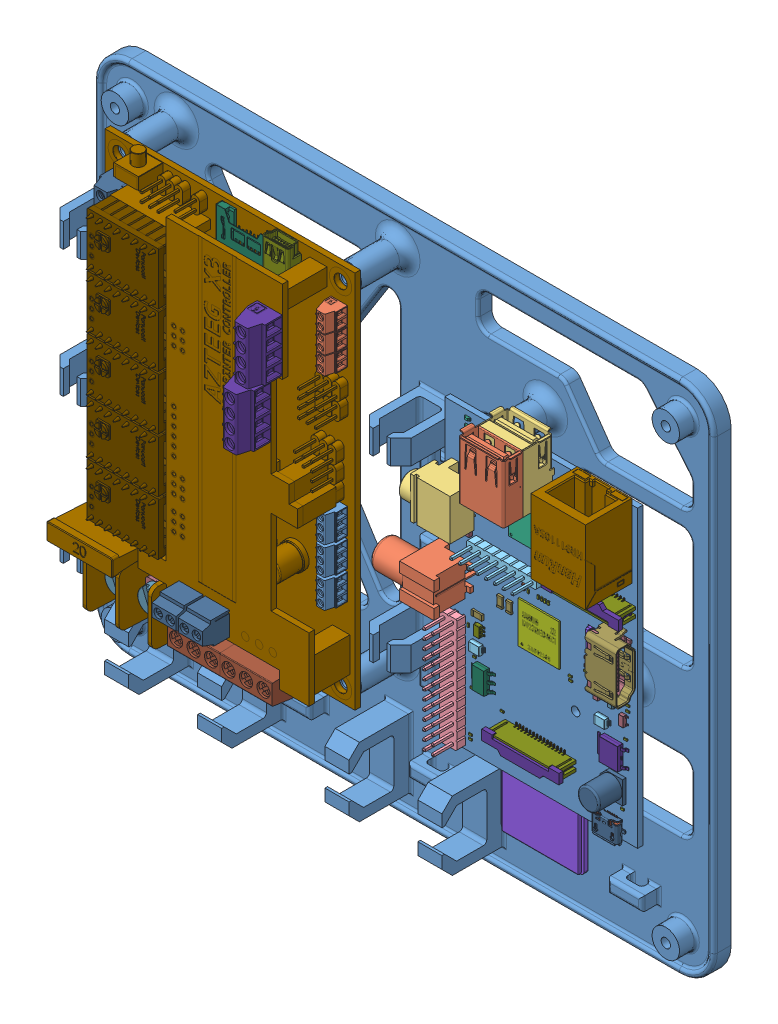
SolidWorks assembly Electronics_Package2, configuration Default. Lengths in mm.
Overall size (180 150 42.6).
296 component instances, 56 part files, 6 mates.
Components (placement in the parent):
- Electronics_Mount-1: Electronics_Mount [Default] at origin size (180 150 22)
- PARASOLID_raspberrypi_b_assembly_mounting_holes-1: PARASOLID_raspberrypi_b_assembly_mounting_holes [Default] at (55.4 9.4 19) x (0 1 0) z (0 0 1) size (110.83 65.9 20.48)
  - raspberry_pi__USB_x2-1: raspberry_pi__USB_x2 [Default] at (41.25 117.3116 21.0675) x (0 1 0) z (1 0 0) size (14.7 17.85 17.4)
    - raspberry_pi__USB_x2_part1-1: raspberry_pi__USB_x2_part1 [Default] at (-114.6616 -10.9375 -4.85) x (0 0 1) z (-1 0 0) size (17.4 6.35 14.7)
    - raspberry_pi__USB_x2_part2-1: raspberry_pi__USB_x2_part2 [Default] at (-114.6616 -19.4375 -4.85) x (0 0 1) z (-1 0 0) size (17.4 11.5 14.7)
  - raspberry_pi__SD_reader_assembly-1: raspberry_pi__SD_reader_assembly [Default] at (-46.9946 70.3951 -2.1406) x (0 1 0) z (-1 0 0) size (32.3 4.2 18.72)
    - raspberry_pi__SD_reader_body-1: raspberry_pi__SD_reader_body [Default] at (-67.8965 -2.1406 21.2643) size (32.3 4.2 16.75)
    - raspberry_pi__SD_reader_pin1-1: raspberry_pi__SD_reader_pin1 [Default] at (-66.0305 -2.1406 -4.4304) x (0 0 -1) z (1 0 0) size (9.85 2.04 0.6)
    - raspberry_pi__SD_reader_pin1-2: raspberry_pi__SD_reader_pin1 [Default] at (-68.5305 -2.1406 -4.4304) x (0 0 -1) z (1 0 0) size (9.85 2.04 0.6)
    - raspberry_pi__SD_reader_pin2-1: raspberry_pi__SD_reader_pin2 [Default] at (-79.4655 -2.1385 -5.3387) x (0 0 -1) z (1 0 0) size (8.94 2.04 0.6)
    - raspberry_pi__SD_reader_pin2-2: raspberry_pi__SD_reader_pin2 [Default] at (-56.8355 -2.1385 -5.3387) x (0 0 -1) z (1 0 0) size (8.94 2.04 0.6)
    - raspberry_pi__SD_reader_pin2-3: raspberry_pi__SD_reader_pin2 [Default] at (-76.0205 -2.1385 -5.3387) x (0 0 -1) z (1 0 0) size (8.94 2.04 0.6)
    - raspberry_pi__SD_reader_pin2-4: raspberry_pi__SD_reader_pin2 [Default] at (-73.5205 -2.1385 -5.3387) x (0 0 -1) z (1 0 0) size (8.94 2.04 0.6)
    - raspberry_pi__SD_reader_pin2-5: raspberry_pi__SD_reader_pin2 [Default] at (-63.5205 -2.1385 -5.3387) x (0 0 -1) z (1 0 0) size (8.94 2.04 0.6)
    - raspberry_pi__SD_reader_pin2-6: raspberry_pi__SD_reader_pin2 [Default] at (-77.6455 -2.1385 -5.3387) x (0 0 -1) z (1 0 0) size (8.94 2.04 0.6)
    - raspberry_pi__SD_reader_pin2-7: raspberry_pi__SD_reader_pin2 [Default] at (-81.1155 -2.1385 -5.3387) x (0 0 -1) z (1 0 0) size (8.94 2.04 0.6)
    - raspberry_pi__SD_reader_pin2-8: raspberry_pi__SD_reader_pin2 [Default] at (-55.3955 -2.1385 -5.3387) x (0 0 -1) z (1 0 0) size (8.94 2.04 0.6)
    - raspberry_pi__SD_reader_pin2-9: raspberry_pi__SD_reader_pin2 [Default] at (-71.0205 -2.1385 -5.3387) x (0 0 -1) z (1 0 0) size (8.94 2.04 0.6)
    - raspberry_pi__SD_reader_pin2-10: raspberry_pi__SD_reader_pin2 [Default] at (-61.0205 -2.1385 -5.3387) x (0 0 -1) z (1 0 0) size (8.94 2.04 0.6)
    - raspberry_pi__SD_reader_pin3-1: raspberry_pi__SD_reader_pin3 [Default] at (-58.5401 -2.1448 -2.5387) x (0 0 -1) z (1 0 0) size (11.74 2.04 0.6)
    - raspberry_pi__SD_reader_pin4-1: raspberry_pi__SD_reader_pin4 [Default] at (-62.6615 0.5594 -20.2143) x (1 0 0) z (0 1 0) size (13.35 0.4 0.55)
    - raspberry_pi__SD_reader_pin5-1: raspberry_pi__SD_reader_pin5 [Default] at (-67.8965 0.5594 -4.5143) x (1 0 0) z (0 1 0) size (13.67 2.63 0.55)
  - raspberry_pi__micro_USB-1: raspberry_pi__micro_USB [Default] at (-58.8764 -35.1801 -3.6369) x (0 -1 0) z (-1 0 0) size (7.97 2.92 5.43)
    - raspberry_pi__micro_USB_cover-1: raspberry_pi__micro_USB_cover [Default] at (-14.4796 6.4719 -16.0085) size (7.97 2.92 5.43)
    - raspberry_pi__micro_USB_contacts-1: raspberry_pi__micro_USB_contacts [Default] at (-14.4796 6.4719 -20.7085) size (6.9 2.16 4.2)
  - raspberry_pi__HDMI_socket-1: raspberry_pi__HDMI_socket [Default] at (2.2003 -19.6809 5.025) x (1 0 0) z (0 -1 0) size (16.2 8 9.9)
    - raspberry_pi__HDMI_socket_cover-1: raspberry_pi__HDMI_socket_cover [Default] at (-20 0 0) size (16.2 8 9)
    - raspberry_pi__HDMI_socket_inside-1: raspberry_pi__HDMI_socket_inside [Default] at (-20 0 0) size (15 6.1 7.6)
    - raspberry_pi__HDMI_socket_large_pin-1: raspberry_pi__HDMI_socket_large_pin [Default] at (-210.7661 0.45 76.5103) x (0 0 -1) z (0 -1 0) size (7.55 0.65 3.84)
    - raspberry_pi__HDMI_socket_large_pin-2: raspberry_pi__HDMI_socket_large_pin [Default] at (-203.7661 0.45 76.5103) x (0 0 -1) z (0 -1 0) size (7.55 0.65 3.84)
    - raspberry_pi__HDMI_socket_large_pin-3: raspberry_pi__HDMI_socket_large_pin [Default] at (-205.7661 0.45 76.5103) x (0 0 -1) z (0 -1 0) size (7.55 0.65 3.84)
    - raspberry_pi__HDMI_socket_large_pin-4: raspberry_pi__HDMI_socket_large_pin [Default] at (-207.7661 0.45 76.5103) x (0 0 -1) z (0 -1 0) size (7.55 0.65 3.84)
    - raspberry_pi__HDMI_socket_large_pin-5: raspberry_pi__HDMI_socket_large_pin [Default] at (-209.7661 0.45 76.5103) x (0 0 -1) z (0 -1 0) size (7.55 0.65 3.84)
    - raspberry_pi__HDMI_socket_large_pin-6: raspberry_pi__HDMI_socket_large_pin [Default] at (-201.7661 0.45 76.5103) x (0 0 -1) z (0 -1 0) size (7.55 0.65 3.84)
    - raspberry_pi__HDMI_socket_large_pin-7: raspberry_pi__HDMI_socket_large_pin [Default] at (-202.7661 0.45 76.5103) x (0 0 -1) z (0 -1 0) size (7.55 0.65 3.84)
    - raspberry_pi__HDMI_socket_large_pin-8: raspberry_pi__HDMI_socket_large_pin [Default] at (-204.7661 0.45 76.5103) x (0 0 -1) z (0 -1 0) size (7.55 0.65 3.84)
    - raspberry_pi__HDMI_socket_large_pin-9: raspberry_pi__HDMI_socket_large_pin [Default] at (-206.7661 0.45 76.5103) x (0 0 -1) z (0 -1 0) size (7.55 0.65 3.84)
    - raspberry_pi__HDMI_socket_large_pin-10: raspberry_pi__HDMI_socket_large_pin [Default] at (-208.7661 0.45 76.5103) x (0 0 -1) z (0 -1 0) size (7.55 0.65 3.84)
    - raspberry_pi__HDMI_socket_small_pin-1: raspberry_pi__HDMI_socket_small_pin [Default] at (-204.2661 -0.25 76.5103) x (0 0 -1) z (0 -1 0) size (7.55 0.65 3.08)
    - raspberry_pi__HDMI_socket_small_pin-2: raspberry_pi__HDMI_socket_small_pin [Default] at (-206.2661 -0.25 76.5103) x (0 0 -1) z (0 -1 0) size (7.55 0.65 3.08)
    - raspberry_pi__HDMI_socket_small_pin-3: raspberry_pi__HDMI_socket_small_pin [Default] at (-208.2661 -0.25 76.5103) x (0 0 -1) z (0 -1 0) size (7.55 0.65 3.08)
    - raspberry_pi__HDMI_socket_small_pin-4: raspberry_pi__HDMI_socket_small_pin [Default] at (-210.2661 -0.25 76.5103) x (0 0 -1) z (0 -1 0) size (7.55 0.65 3.08)
    - raspberry_pi__HDMI_socket_small_pin-5: raspberry_pi__HDMI_socket_small_pin [Default] at (-203.2661 -0.25 76.5103) x (0 0 -1) z (0 -1 0) size (7.55 0.65 3.08)
    - raspberry_pi__HDMI_socket_small_pin-6: raspberry_pi__HDMI_socket_small_pin [Default] at (-205.2661 -0.25 76.5103) x (0 0 -1) z (0 -1 0) size (7.55 0.65 3.08)
    - raspberry_pi__HDMI_socket_small_pin-7: raspberry_pi__HDMI_socket_small_pin [Default] at (-207.2661 -0.25 76.5103) x (0 0 -1) z (0 -1 0) size (7.55 0.65 3.08)
    - raspberry_pi__HDMI_socket_small_pin-8: raspberry_pi__HDMI_socket_small_pin [Default] at (-209.2661 -0.25 76.5103) x (0 0 -1) z (0 -1 0) size (7.55 0.65 3.08)
    - raspberry_pi__HDMI_socket_small_pin-9: raspberry_pi__HDMI_socket_small_pin [Default] at (-202.2661 -0.25 76.5103) x (0 0 -1) z (0 -1 0) size (7.55 0.65 3.08)
  - raspberry_pi__15_pin_FFC_Connector-1: raspberry_pi__15_pin_FFC_Connector [Default] at (69.3611 0.0667 -17.4242) x (1 0 0) z (0 -1 0) size (4.85 6 22.4)
    - raspberry_pi__15_pin_FFC_Connector_body-1: raspberry_pi__15_pin_FFC_Connector_body [Default] at (-100.5372 19.1242 0) size (2.9 5.7 20.6)
    - raspberry_pi__15_pin_FFC_Connector_locker-1: raspberry_pi__15_pin_FFC_Connector_locker [Default] at (-101.0372 23.8242 0) size (4 5.4 22.4)
    - raspberry_pi__15_pin_FFC_Connector_pins-1: raspberry_pi__15_pin_FFC_Connector_pins [Default] at (-100.5372 19.1242 -0.85) x (-1 0 0) z (0 0 -1) size (4.3 4.71 0.3)
    - raspberry_pi__15_pin_FFC_Connector_pins-2: raspberry_pi__15_pin_FFC_Connector_pins [Default] at (-100.5372 19.1242 5.15) x (-1 0 0) z (0 0 -1) size (4.3 4.71 0.3)
    - raspberry_pi__15_pin_FFC_Connector_pins-3: raspberry_pi__15_pin_FFC_Connector_pins [Default] at (-100.5372 19.1242 -1.85) x (-1 0 0) z (0 0 -1) size (4.3 4.71 0.3)
    - raspberry_pi__15_pin_FFC_Connector_pins-4: raspberry_pi__15_pin_FFC_Connector_pins [Default] at (-100.5372 19.1242 4.15) x (-1 0 0) z (0 0 -1) size (4.3 4.71 0.3)
    - raspberry_pi__15_pin_FFC_Connector_pins-5: raspberry_pi__15_pin_FFC_Connector_pins [Default] at (-100.5372 19.1242 -2.85) x (-1 0 0) z (0 0 -1) size (4.3 4.71 0.3)
    - raspberry_pi__15_pin_FFC_Connector_pins-6: raspberry_pi__15_pin_FFC_Connector_pins [Default] at (-100.5372 19.1242 3.15) x (-1 0 0) z (0 0 -1) size (4.3 4.71 0.3)
    - raspberry_pi__15_pin_FFC_Connector_pins-7: raspberry_pi__15_pin_FFC_Connector_pins [Default] at (-100.5372 19.1242 -3.85) x (-1 0 0) z (0 0 -1) size (4.3 4.71 0.3)
    - raspberry_pi__15_pin_FFC_Connector_pins-8: raspberry_pi__15_pin_FFC_Connector_pins [Default] at (-100.5372 19.1242 2.15) x (-1 0 0) z (0 0 -1) size (4.3 4.71 0.3)
    - raspberry_pi__15_pin_FFC_Connector_pins-9: raspberry_pi__15_pin_FFC_Connector_pins [Default] at (-100.5372 19.1242 -4.85) x (-1 0 0) z (0 0 -1) size (4.3 4.71 0.3)
    - raspberry_pi__15_pin_FFC_Connector_pins-10: raspberry_pi__15_pin_FFC_Connector_pins [Default] at (-100.5372 19.1242 1.15) x (-1 0 0) z (0 0 -1) size (4.3 4.71 0.3)
    - raspberry_pi__15_pin_FFC_Connector_pins-11: raspberry_pi__15_pin_FFC_Connector_pins [Default] at (-100.5372 19.1242 7.15) x (-1 0 0) z (0 0 -1) size (4.3 4.71 0.3)
    - raspberry_pi__15_pin_FFC_Connector_pins-12: raspberry_pi__15_pin_FFC_Connector_pins [Default] at (-100.5372 19.1242 -5.85) x (-1 0 0) z (0 0 -1) size (4.3 4.71 0.3)
    - raspberry_pi__15_pin_FFC_Connector_pins-13: raspberry_pi__15_pin_FFC_Connector_pins [Default] at (-100.5372 19.1242 0.15) x (-1 0 0) z (0 0 -1) size (4.3 4.71 0.3)
    - raspberry_pi__15_pin_FFC_Connector_pins-14: raspberry_pi__15_pin_FFC_Connector_pins [Default] at (-100.5372 19.1242 6.15) x (-1 0 0) z (0 0 -1) size (4.3 4.71 0.3)
    - raspberry_pi__15_pin_FFC_Connector_pins-15: raspberry_pi__15_pin_FFC_Connector_pins [Default] at (-100.5372 19.1242 -6.85) x (-1 0 0) z (0 0 -1) size (4.3 4.71 0.3)
  - raspberry_pi__15_pin_FFC_Connector-1-1: raspberry_pi__15_pin_FFC_Connector-1 [Default] at (-84.4423 -17.203 -17.4242) x (-1 0 0) z (0 1 0) size (4.85 6 22.4)
    - raspberry_pi__15_pin_FFC_Connector_body-1: raspberry_pi__15_pin_FFC_Connector_body [Default] at (-100.5372 19.1242 0) size (2.9 5.7 20.6)
    - raspberry_pi__15_pin_FFC_Connector_locker-1: raspberry_pi__15_pin_FFC_Connector_locker [Default] at (-101.0372 23.8242 0) size (4 5.4 22.4)
    - raspberry_pi__15_pin_FFC_Connector_pins-1: raspberry_pi__15_pin_FFC_Connector_pins [Default] at (-100.5372 19.1242 7.15) x (-1 0 0) z (0 0 -1) size (4.3 4.71 0.3)
    - raspberry_pi__15_pin_FFC_Connector_pins-2: raspberry_pi__15_pin_FFC_Connector_pins [Default] at (-100.5372 19.1242 0.15) x (-1 0 0) z (0 0 -1) size (4.3 4.71 0.3)
    - raspberry_pi__15_pin_FFC_Connector_pins-3: raspberry_pi__15_pin_FFC_Connector_pins [Default] at (-100.5372 19.1242 -6.85) x (-1 0 0) z (0 0 -1) size (4.3 4.71 0.3)
    - raspberry_pi__15_pin_FFC_Connector_pins-4: raspberry_pi__15_pin_FFC_Connector_pins [Default] at (-100.5372 19.1242 6.15) x (-1 0 0) z (0 0 -1) size (4.3 4.71 0.3)
    - raspberry_pi__15_pin_FFC_Connector_pins-5: raspberry_pi__15_pin_FFC_Connector_pins [Default] at (-100.5372 19.1242 -0.85) x (-1 0 0) z (0 0 -1) size (4.3 4.71 0.3)
    - raspberry_pi__15_pin_FFC_Connector_pins-6: raspberry_pi__15_pin_FFC_Connector_pins [Default] at (-100.5372 19.1242 5.15) x (-1 0 0) z (0 0 -1) size (4.3 4.71 0.3)
    - raspberry_pi__15_pin_FFC_Connector_pins-7: raspberry_pi__15_pin_FFC_Connector_pins [Default] at (-100.5372 19.1242 -1.85) x (-1 0 0) z (0 0 -1) size (4.3 4.71 0.3)
    - raspberry_pi__15_pin_FFC_Connector_pins-8: raspberry_pi__15_pin_FFC_Connector_pins [Default] at (-100.5372 19.1242 4.15) x (-1 0 0) z (0 0 -1) size (4.3 4.71 0.3)
    - raspberry_pi__15_pin_FFC_Connector_pins-9: raspberry_pi__15_pin_FFC_Connector_pins [Default] at (-100.5372 19.1242 -2.85) x (-1 0 0) z (0 0 -1) size (4.3 4.71 0.3)
    - raspberry_pi__15_pin_FFC_Connector_pins-10: raspberry_pi__15_pin_FFC_Connector_pins [Default] at (-100.5372 19.1242 3.15) x (-1 0 0) z (0 0 -1) size (4.3 4.71 0.3)
    - raspberry_pi__15_pin_FFC_Connector_pins-11: raspberry_pi__15_pin_FFC_Connector_pins [Default] at (-100.5372 19.1242 -3.85) x (-1 0 0) z (0 0 -1) size (4.3 4.71 0.3)
    - raspberry_pi__15_pin_FFC_Connector_pins-12: raspberry_pi__15_pin_FFC_Connector_pins [Default] at (-100.5372 19.1242 2.15) x (-1 0 0) z (0 0 -1) size (4.3 4.71 0.3)
    - raspberry_pi__15_pin_FFC_Connector_pins-13: raspberry_pi__15_pin_FFC_Connector_pins [Default] at (-100.5372 19.1242 -4.85) x (-1 0 0) z (0 0 -1) size (4.3 4.71 0.3)
    - raspberry_pi__15_pin_FFC_Connector_pins-14: raspberry_pi__15_pin_FFC_Connector_pins [Default] at (-100.5372 19.1242 1.15) x (-1 0 0) z (0 0 -1) size (4.3 4.71 0.3)
    - raspberry_pi__15_pin_FFC_Connector_pins-15: raspberry_pi__15_pin_FFC_Connector_pins [Default] at (-100.5372 19.1242 -5.85) x (-1 0 0) z (0 0 -1) size (4.3 4.71 0.3)
  - raspberry_pi__CI_Board_mounting_holes-1: raspberry_pi__CI_Board_mounting_holes [Default] at origin size (85.6 56 1.6)
  - raspberry_pi__composite_video_out-1: raspberry_pi__composite_video_out [Default] at (2.8 18 9.75) x (0 1 0) z (1 0 0) size (19.5 15 10)
  - raspberry_pi__audio_out-1: raspberry_pi__audio_out [Default] at (22.2 31.5 8.1) x (0 1 0) z (0 0 1) size (15 12 14.24)
  - raspberry_pi__bar_180_2x13-1: raspberry_pi__bar_180_2x13 [Default] at (-41.124 25.7906 4.1) x (0 1 0) z (-1 0 0) size (5.08 11.6 33.02)
  - raspberry_pi__bar_180_1x8-1: raspberry_pi__bar_180_1x8 [Default] at (10.9423 17.9314 4.1) x (1 0 0) z (0 1 0) size (2.54 12.5 20.32)
  - raspberry_pi__QFN64-2-1: raspberry_pi__QFN64-2 [Default] at (22.1224 4.1003 1.6) x (0 -1 0) z (-1 0 0) size (9.04 0.9 9.04)
  - raspberry_pi__168_FBGA_12x12-1: raspberry_pi__168_FBGA_12x12 [Default] at (-2.8005 0.0828 1.87) size (12 12 0.71)
  - raspberry_pi__SD Card-1: raspberry_pi__SD Card [Default] at (-28.7303 2.5002 -1.65) x (0 1 0) z (0 0 -1) size (24 32.02 2.12)
  - raspberry_pi__RJ45-1: raspberry_pi__RJ45 [Default] at (44.2147 -26.3896 15.1) x (0 1 0) z (1 0 0) size (15.88 16.5 21.4)
  - raspberry_pi__capacitor_smd-1: raspberry_pi__capacitor_smd [Default] at (-30.3077 -21.3541 1.6) x (1 0 0) z (0 -1 0) size (6.6 7.7 6.6)
  - raspberry_pi__0603-1: raspberry_pi__0603 [Default] at (-20.0168 3.0701 -0.2285) x (1 0 0) z (0 -1 0) size (1.52 0.46 0.77)
  - raspberry_pi__0603-2: raspberry_pi__0603 [Default] at (30.15 5.1655 1.8285) x (0 -1 0) z (-1 0 0) size (1.52 0.46 0.77)
  - raspberry_pi__0603-3: raspberry_pi__0603 [Default] at (-11.1399 1.5383 -0.2285) x (1 0 0) z (0 -1 0) size (1.52 0.46 0.77)
  - raspberry_pi__0603-4: raspberry_pi__0603 [Default] at (-4.3204 -13.62 1.8285) x (0 -1 0) z (-1 0 0) size (1.52 0.46 0.77)
  - raspberry_pi__0603-5: raspberry_pi__0603 [Default] at (4.3527 1.8422 -0.2285) x (1 0 0) z (0 -1 0) size (1.52 0.46 0.77)
  - raspberry_pi__0603-6: raspberry_pi__0603 [Default] at (4.438 5.0146 -0.2285) x (1 0 0) z (0 -1 0) size (1.52 0.46 0.77)
  - raspberry_pi__0603-7: raspberry_pi__0603 [Default] at (30.1638 8.6161 1.8285) x (0 -1 0) z (-1 0 0) size (1.52 0.46 0.77)
  - raspberry_pi__0603-8: raspberry_pi__0603 [Default] at (-5.9869 -2.4205 -0.2285) x (1 0 0) z (0 -1 0) size (1.52 0.46 0.77)
  - raspberry_pi__0603-9: raspberry_pi__0603 [Default] at (15.354 6.8381 -0.2285) x (0 -1 0) z (-1 0 0) size (1.52 0.46 0.77)
  - raspberry_pi__0603-10: raspberry_pi__0603 [Default] at (6.4098 4.87 1.8285) x (1 0 0) z (0 -1 0) size (1.52 0.46 0.77)
  - raspberry_pi__0603-11: raspberry_pi__0603 [Default] at (-2.2676 -13.6378 1.8285) x (0 -1 0) z (-1 0 0) size (1.52 0.46 0.77)
  - raspberry_pi__0603-12: raspberry_pi__0603 [Default] at (16.4777 -2.9981 1.8285) x (1 0 0) z (0 -1 0) size (1.52 0.46 0.77)
  - raspberry_pi__0603-13: raspberry_pi__0603 [Default] at (4.3628 0.0275 -0.2285) x (1 0 0) z (0 -1 0) size (1.52 0.46 0.77)
  - raspberry_pi__0603-14: raspberry_pi__0603 [Default] at (26.0912 -3.0002 1.8285) x (1 0 0) z (0 -1 0) size (1.52 0.46 0.77)
  - raspberry_pi__1206-1: raspberry_pi__1206 [Default] at (0.9117 11.5772 1.6) x (-1 0 0) z (0 0 1) size (3.05 1.53 0.61)
  - raspberry_pi__1206-2: raspberry_pi__1206 [Default] at (27.5206 15.2101 -0.6096) x (0 -1 0) z (0 0 1) size (3.05 1.53 0.61)
  - raspberry_pi__1206-3: raspberry_pi__1206 [Default] at (-37.0878 -25.7251 -0.6096) x (-1 0 0) z (0 0 1) size (3.05 1.53 0.61)
  - raspberry_pi__1206-4: raspberry_pi__1206 [Default] at (-7.2704 19.6988 1.6) x (0 -1 0) z (0 0 1) size (3.05 1.53 0.61)
  - raspberry_pi__1206-5: raspberry_pi__1206 [Default] at (0.8765 8.9453 1.6) x (-1 0 0) z (0 0 1) size (3.05 1.53 0.61)
  - raspberry_pi__1206-6: raspberry_pi__1206 [Default] at (16.4006 15.2101 -0.6096) x (0 -1 0) z (0 0 1) size (3.05 1.53 0.61)
  - raspberry_pi__Sot23-1: raspberry_pi__Sot23 [Default] at (-9.3808 -16.7671 2.0717) x (1 0 0) z (0 -1 0) size (2.9 1.07 2.4)
  - raspberry_pi__Sot23-2: raspberry_pi__Sot23 [Default] at (12.3003 21.3524 2.0717) x (0 1 0) z (1 0 0) size (2.9 1.07 2.4)
  - raspberry_pi__Sot23-3: raspberry_pi__Sot23 [Default] at (2.0602 -23.9435 -0.4717) x (-1 0 0) z (0 -1 0) size (2.9 1.07 2.4)
  - raspberry_pi__Sot23-4: raspberry_pi__Sot23 [Default] at (23.9618 13.6561 -0.4717) x (-1 0 0) z (0 -1 0) size (2.9 1.07 2.4)
  - raspberry_pi__Sot23-5: raspberry_pi__Sot23 [Default] at (-12.4063 -24.1966 2.0717) x (1 0 0) z (0 -1 0) size (2.9 1.07 2.4)
  - raspberry_pi__Sot23-6: raspberry_pi__Sot23 [Default] at (5.9102 -23.9435 -0.4717) x (-1 0 0) z (0 -1 0) size (2.9 1.07 2.4)
  - raspberry_pi__Sot23-7: raspberry_pi__Sot23 [Default] at (-1.7898 -23.9435 -0.4717) x (-1 0 0) z (0 -1 0) size (2.9 1.07 2.4)
  - raspberry_pi__Sot23-8: raspberry_pi__Sot23 [Default] at (19.9118 13.6561 -0.4717) x (-1 0 0) z (0 -1 0) size (2.9 1.07 2.4)
  - raspberry_pi__Smd6-1: raspberry_pi__Smd6 [Default] at (-12.6331 -22.8121 1.7016) size (2.3 3.02 1.45)
  - raspberry_pi__Sot223-1: raspberry_pi__Sot223 [Default] at (-22.454 16.7753 2.3) x (1 0 0) z (0 -1 0) size (6.5 1.9 6.98)
  - raspberry_pi__Sot23-3_5pins-1: raspberry_pi__Sot23-3_5pins [Default] at (-10.7913 17.6996 2.51) x (1 0 0) z (0 -1 0) size (2.92 1.18 2.85)
  - raspberry_pi__sot-223_large-1: raspberry_pi__sot-223_large [Default] at (-22.0626 -21.058 2.3625) x (1 0 0) z (0 -1 0) size (6.5 1.68 8.93)
  - raspberry_pi__Xtal_Smd_25-1: raspberry_pi__Xtal_Smd_25 [Default] at (21.5599 -6.0522 -0.05) x (1 0 0) z (0 1 0) size (6.5 1.27 4.5)
  - raspberry_pi__1206xl-1: raspberry_pi__1206xl [Default] at (-2.7879 7.0598 -0.6096) x (0 1 0) z (0 0 1) size (3.05 2.04 0.61)
  - raspberry_pi__Xtal_Smd_19200-1: raspberry_pi__Xtal_Smd_19200 [Default] at (-2.6964 -10.154 -0.05) x (0 -1 0) z (1 0 0) size (6.5 1.27 4.5)
  - raspberry_pi__1210-1: raspberry_pi__1210 [Default] at (-27.0775 -21.3756 -0.85) x (0 1 0) z (0 0 1) size (3.2 2.49 1.7)
  - raspberry_pi__1812-1: raspberry_pi__1812 [Default] at (31.1876 15.6132 1.6) x (0 -1 0) z (0 0 1) size (4.74 3.48 1.04)
  - raspberry_pi__1812-2: raspberry_pi__1812 [Default] at (-33.1773 -21.181 0) x (0 -1 0) z (0 0 -1) size (4.74 3.48 1.04)
  - raspberry_pi__SOD-123_DiodesInc-1: raspberry_pi__SOD-123_DiodesInc [Default] at (-16.6177 19.8007 2.025) x (0 -1 0) z (0 0 1) size (4.1 2.5 1.45)
  - raspberry_pi__SOD-123_DiodesInc-2: raspberry_pi__SOD-123_DiodesInc [Default] at (-16.7495 -16.6513 2.025) x (0 -1 0) z (0 0 1) size (4.1 2.5 1.45)
  - raspberry_pi__LED_SMD_0603-1: raspberry_pi__LED_SMD_0603 [Default] at (37.4435 21.7741 1.6) size (0.73 1.65 0.68)
  - raspberry_pi__LED_SMD_0603-2: raspberry_pi__LED_SMD_0603 [Default] at (35.4303 21.8177 1.6) size (0.73 1.65 0.68)
  - raspberry_pi__LED_SMD_0603-3: raspberry_pi__LED_SMD_0603 [Default] at (30.4163 21.764 1.6) size (0.73 1.65 0.68)
  - raspberry_pi__LED_SMD_0603-4: raspberry_pi__LED_SMD_0603 [Default] at (39.4716 21.7671 1.6) size (0.73 1.65 0.68)
  - raspberry_pi__LED_SMD_0603-5: raspberry_pi__LED_SMD_0603 [Default] at (32.4024 21.8003 1.6) size (0.73 1.65 0.68)
  - raspberry_pi__0402-1: raspberry_pi__0402 [Default] at (16.5111 -5.5807 0) x (0 1 0) z (0 0 -1) size (1 0.5 0.3)
  - raspberry_pi__0402-2: raspberry_pi__0402 [Default] at (26.6197 -6.5224 0) x (0 1 0) z (0 0 -1) size (1 0.5 0.3)
  - raspberry_pi__0402-3: raspberry_pi__0402 [Default] at (26.6409 2.5469 0) x (-1 0 0) z (0 0 -1) size (1 0.5 0.3)
  - raspberry_pi__0402-4: raspberry_pi__0402 [Default] at (26.5831 4.5716 0) x (-1 0 0) z (0 0 -1) size (1 0.5 0.3)
  - raspberry_pi__0402-5: raspberry_pi__0402 [Default] at (-7.9744 2.1558 0) x (-1 0 0) z (0 0 -1) size (1 0.5 0.3)
  - raspberry_pi__0402-6: raspberry_pi__0402 [Default] at (-7.8 -3.8157 0) x (-1 0 0) z (0 0 -1) size (1 0.5 0.3)
  - raspberry_pi__0402-7: raspberry_pi__0402 [Default] at (-5.4305 -5.2325 0) x (-1 0 0) z (0 0 -1) size (1 0.5 0.3)
  - raspberry_pi__0402-8: raspberry_pi__0402 [Default] at (-9.7312 -4.8048 0) x (-1 0 0) z (0 0 -1) size (1 0.5 0.3)
  - raspberry_pi__0402-9: raspberry_pi__0402 [Default] at (30.6617 -5.5228 1.6) size (1 0.5 0.3)
  - raspberry_pi__0402-10: raspberry_pi__0402 [Default] at (-8.5936 -2.8148 0) x (-1 0 0) z (0 0 -1) size (1 0.5 0.3)
  - raspberry_pi__0402-11: raspberry_pi__0402 [Default] at (5.8653 -0.2743 1.6) size (1 0.5 0.3)
  - raspberry_pi__0402-12: raspberry_pi__0402 [Default] at (-20.5335 6.6422 0) x (-1 0 0) z (0 0 -1) size (1 0.5 0.3)
  - raspberry_pi__0402-13: raspberry_pi__0402 [Default] at (30.6048 -2.0048 1.6) size (1 0.5 0.3)
  - raspberry_pi__0402-14: raspberry_pi__0402 [Default] at (4.5867 -5.9499 0) x (-1 0 0) z (0 0 -1) size (1 0.5 0.3)
  - raspberry_pi__0402-15: raspberry_pi__0402 [Default] at (23.1074 -7.0265 1.6) size (1 0.5 0.3)
  - raspberry_pi__0402-16: raspberry_pi__0402 [Default] at (-0.9337 5.6221 0) x (-1 0 0) z (0 0 -1) size (1 0.5 0.3)
  - raspberry_pi__0402-17: raspberry_pi__0402 [Default] at (20.4385 -13.9007 1.6) size (1 0.5 0.3)
  - raspberry_pi__0402-18: raspberry_pi__0402 [Default] at (17.5415 -0.013 0) x (-1 0 0) z (0 0 -1) size (1 0.5 0.3)
  - raspberry_pi__0402-19: raspberry_pi__0402 [Default] at (20.3971 -16.3895 1.6) size (1 0.5 0.3)
  - raspberry_pi__0402-20: raspberry_pi__0402 [Default] at (26.5926 5.5414 0) x (-1 0 0) z (0 0 -1) size (1 0.5 0.3)
  - raspberry_pi__0402-21: raspberry_pi__0402 [Default] at (20.3928 -17.7386 1.6) size (1 0.5 0.3)
  - raspberry_pi__0402-22: raspberry_pi__0402 [Default] at (28.6241 9.1278 1.6) x (0 1 0) z (0 0 1) size (1 0.5 0.3)
  - raspberry_pi__0402-23: raspberry_pi__0402 [Default] at (26.5896 7.0878 0) x (-1 0 0) z (0 0 -1) size (1 0.5 0.3)
  - raspberry_pi__0402-24: raspberry_pi__0402 [Default] at (20.4147 -21.2973 1.6) size (1 0.5 0.3)
  - raspberry_pi__0402-25: raspberry_pi__0402 [Default] at (36.5484 22.6274 0) x (0 1 0) z (0 0 -1) size (1 0.5 0.3)
  - raspberry_pi__0402-26: raspberry_pi__0402 [Default] at (23.7892 -2.5954 0) x (-1 0 0) z (0 0 -1) size (1 0.5 0.3)
  - raspberry_pi__0402-27: raspberry_pi__0402 [Default] at (20.4617 -22.8315 1.6) size (1 0.5 0.3)
  - raspberry_pi__0402-28: raspberry_pi__0402 [Default] at (20.5208 -0.5268 0) x (0 1 0) z (0 0 -1) size (1 0.5 0.3)
  - raspberry_pi__0402-29: raspberry_pi__0402 [Default] at (2.5305 6.5943 0) x (-1 0 0) z (0 0 -1) size (1 0.5 0.3)
  - raspberry_pi__0402-30: raspberry_pi__0402 [Default] at (16.5404 -1.0094 0) x (-1 0 0) z (0 0 -1) size (1 0.5 0.3)
  - raspberry_pi__0402-31: raspberry_pi__0402 [Default] at (20.0197 14.6983 1.6) x (0 1 0) z (0 0 1) size (1 0.5 0.3)
  - raspberry_pi__0402-32: raspberry_pi__0402 [Default] at (-0.2126 6.608 0) x (-1 0 0) z (0 0 -1) size (1 0.5 0.3)
  - raspberry_pi__0402-33: raspberry_pi__0402 [Default] at (14.5614 -22.3029 0) x (-1 0 0) z (0 0 -1) size (1 0.5 0.3)
  - raspberry_pi__0402-34: raspberry_pi__0402 [Default] at (24.6737 14.716 1.6) x (0 1 0) z (0 0 1) size (1 0.5 0.3)
  - raspberry_pi__0402-35: raspberry_pi__0402 [Default] at (2.3756 -1.7794 0) x (-1 0 0) z (0 0 -1) size (1 0.5 0.3)
  - raspberry_pi__0402-36: raspberry_pi__0402 [Default] at (14.5643 -23.2503 0) x (-1 0 0) z (0 0 -1) size (1 0.5 0.3)
  - raspberry_pi__0402-37: raspberry_pi__0402 [Default] at (-18.4181 19.2242 1.6) x (0 1 0) z (0 0 1) size (1 0.5 0.3)
  - raspberry_pi__0402-38: raspberry_pi__0402 [Default] at (3.9214 -4.1571 0) x (-1 0 0) z (0 0 -1) size (1 0.5 0.3)
  - raspberry_pi__0402-39: raspberry_pi__0402 [Default] at (14.5643 -24.2749 0) x (-1 0 0) z (0 0 -1) size (1 0.5 0.3)
  - raspberry_pi__0402-40: raspberry_pi__0402 [Default] at (-5.8382 -13.1063 1.6) x (0 1 0) z (0 0 1) size (1 0.5 0.3)
  - raspberry_pi__0402-41: raspberry_pi__0402 [Default] at (-2.5739 3.9906 0) x (-1 0 0) z (0 0 -1) size (1 0.5 0.3)
  - raspberry_pi__0402-42: raspberry_pi__0402 [Default] at (-39.7276 20.3967 1.6) x (0 1 0) z (0 0 1) size (1 0.5 0.3)
  - raspberry_pi__0402-43: raspberry_pi__0402 [Default] at (-10.4678 -8.6884 1.6) x (0 1 0) z (0 0 1) size (1 0.5 0.3)
  - raspberry_pi__0402-44: raspberry_pi__0402 [Default] at (-7.9084 3.2813 0) x (-1 0 0) z (0 0 -1) size (1 0.5 0.3)
  - raspberry_pi__0402-45: raspberry_pi__0402 [Default] at (-11.3406 21.073 1.6) size (1 0.5 0.3)
  - raspberry_pi__0402-46: raspberry_pi__0402 [Default] at (-35.7319 -1.5438 1.6) x (0 1 0) z (0 0 1) size (1 0.5 0.3)
  - raspberry_pi__0402-47: raspberry_pi__0402 [Default] at (-8.6287 -0.7468 0) x (-1 0 0) z (0 0 -1) size (1 0.5 0.3)
  - raspberry_pi__0402-48: raspberry_pi__0402 [Default] at (-33.7587 -16.4954 1.6) size (1 0.5 0.3)
  - raspberry_pi__0402-49: raspberry_pi__0402 [Default] at (-28.0813 11.1601 1.6) x (0 1 0) z (0 0 1) size (1 0.5 0.3)
  - raspberry_pi__0402-50: raspberry_pi__0402 [Default] at (-0.1693 -20.7251 0) x (-1 0 0) z (0 0 -1) size (1 0.5 0.3)
  - raspberry_pi__0402-51: raspberry_pi__0402 [Default] at (5.8711 3.5923 1.6) size (1 0.5 0.3)
  - raspberry_pi__0402-52: raspberry_pi__0402 [Default] at (-35.2523 -23.7657 1.6) x (0 1 0) z (0 0 1) size (1 0.5 0.3)
  - raspberry_pi__0402-53: raspberry_pi__0402 [Default] at (-10.175 0.2473 0) x (-1 0 0) z (0 0 -1) size (1 0.5 0.3)
  - raspberry_pi__0402-54: raspberry_pi__0402 [Default] at (5.8661 -2.2763 1.6) size (1 0.5 0.3)
  - raspberry_pi__0402-55: raspberry_pi__0402 [Default] at (26.0716 14.711 1.6) x (0 1 0) z (0 0 1) size (1 0.5 0.3)
  - raspberry_pi__0402-56: raspberry_pi__0402 [Default] at (1.8359 0.022 0) x (-1 0 0) z (0 0 -1) size (1 0.5 0.3)
  - raspberry_pi__0402-57: raspberry_pi__0402 [Default] at (5.862 -1.271 1.6) size (1 0.5 0.3)
  - raspberry_pi__0402-58: raspberry_pi__0402 [Default] at (24.6779 12.4161 1.6) x (0 1 0) z (0 0 1) size (1 0.5 0.3)
  - raspberry_pi__0402-59: raspberry_pi__0402 [Default] at (1.7944 1.3423 0) x (-1 0 0) z (0 0 -1) size (1 0.5 0.3)
  - raspberry_pi__0402-60: raspberry_pi__0402 [Default] at (5.8694 0.7123 1.6) size (1 0.5 0.3)
  - raspberry_pi__0402-61: raspberry_pi__0402 [Default] at (18.6901 14.7017 1.6) x (0 1 0) z (0 0 1) size (1 0.5 0.3)
  - raspberry_pi__0402-62: raspberry_pi__0402 [Default] at (1.7432 3.7872 0) x (-1 0 0) z (0 0 -1) size (1 0.5 0.3)
  - raspberry_pi__0402-63: raspberry_pi__0402 [Default] at (20.4286 -12.9189 1.6) size (1 0.5 0.3)
  - raspberry_pi__0402-64: raspberry_pi__0402 [Default] at (20.0417 12.4795 1.6) x (0 1 0) z (0 0 1) size (1 0.5 0.3)
  - raspberry_pi__0402-65: raspberry_pi__0402 [Default] at (17.5629 0.9622 0) x (-1 0 0) z (0 0 -1) size (1 0.5 0.3)
  - raspberry_pi__0402-66: raspberry_pi__0402 [Default] at (20.8033 -7.0109 1.6) size (1 0.5 0.3)
  - raspberry_pi__0402-67: raspberry_pi__0402 [Default] at (40.4946 22.5794 0) x (0 1 0) z (0 0 -1) size (1 0.5 0.3)
  - raspberry_pi__0402-68: raspberry_pi__0402 [Default] at (17.5434 4.0775 0) x (-1 0 0) z (0 0 -1) size (1 0.5 0.3)
  - raspberry_pi__0402-69: raspberry_pi__0402 [Default] at (19.1625 -6.0173 1.6) size (1 0.5 0.3)
  - raspberry_pi__0402-70: raspberry_pi__0402 [Default] at (21.5231 -0.5052 0) x (0 1 0) z (0 0 -1) size (1 0.5 0.3)
  - raspberry_pi__0402-71: raspberry_pi__0402 [Default] at (17.4989 5.4204 0) x (-1 0 0) z (0 0 -1) size (1 0.5 0.3)
  - raspberry_pi__0402-72: raspberry_pi__0402 [Default] at (21.4628 -6.0814 1.6) size (1 0.5 0.3)
  - raspberry_pi__0402-73: raspberry_pi__0402 [Default] at (25.1155 -0.5281 0) x (0 1 0) z (0 0 -1) size (1 0.5 0.3)
  - raspberry_pi__0402-74: raspberry_pi__0402 [Default] at (3.4364 -20.7631 0) x (-1 0 0) z (0 0 -1) size (1 0.5 0.3)
  - raspberry_pi__0402-75: raspberry_pi__0402 [Default] at (-38.5189 20.3851 1.6) x (0 1 0) z (0 0 1) size (1 0.5 0.3)
  - raspberry_pi__0402-76: raspberry_pi__0402 [Default] at (29.152 2.0484 0) x (0 1 0) z (0 0 -1) size (1 0.5 0.3)
  - raspberry_pi__0402-77: raspberry_pi__0402 [Default] at (-4.6525 -1.1002 0) x (-1 0 0) z (0 0 -1) size (1 0.5 0.3)
  - raspberry_pi__0402-78: raspberry_pi__0402 [Default] at (-26.5906 19.9445 1.6) x (0 1 0) z (0 0 1) size (1 0.5 0.3)
  - raspberry_pi__0402-79: raspberry_pi__0402 [Default] at (30.1127 2.0467 0) x (0 1 0) z (0 0 -1) size (1 0.5 0.3)
  - raspberry_pi__0402-80: raspberry_pi__0402 [Default] at (-20.5406 8.1106 0) x (-1 0 0) z (0 0 -1) size (1 0.5 0.3)
  - raspberry_pi__0402-81: raspberry_pi__0402 [Default] at (-9.3677 -8.6318 1.6) x (0 1 0) z (0 0 1) size (1 0.5 0.3)
  - raspberry_pi__0402-82: raspberry_pi__0402 [Default] at (26.1021 -0.4966 0) x (0 1 0) z (0 0 -1) size (1 0.5 0.3)
  - raspberry_pi__0402-83: raspberry_pi__0402 [Default] at (8.8247 -0.0532 0) x (-1 0 0) z (0 0 -1) size (1 0.5 0.3)
  - raspberry_pi__0402-84: raspberry_pi__0402 [Default] at (-9.8959 -25.3143 1.6) x (0 1 0) z (0 0 1) size (1 0.5 0.3)
  - raspberry_pi__0402-85: raspberry_pi__0402 [Default] at (20.4897 8.4995 0) x (0 1 0) z (0 0 -1) size (1 0.5 0.3)
  - raspberry_pi__0402-86: raspberry_pi__0402 [Default] at (-5.3787 -3.6334 0) x (-1 0 0) z (0 0 -1) size (1 0.5 0.3)
  - raspberry_pi__0402-87: raspberry_pi__0402 [Default] at (-8.4026 -25.3185 1.6) x (0 1 0) z (0 0 1) size (1 0.5 0.3)
  - raspberry_pi__0402-88: raspberry_pi__0402 [Default] at (25.0176 8.5762 0) x (0 1 0) z (0 0 -1) size (1 0.5 0.3)
  - raspberry_pi__0402-89: raspberry_pi__0402 [Default] at (-5.517 0.0006 0) x (-1 0 0) z (0 0 -1) size (1 0.5 0.3)
  - raspberry_pi__0402-90: raspberry_pi__0402 [Default] at (-17.239 -24.6796 1.6) x (0 1 0) z (0 0 1) size (1 0.5 0.3)
  - raspberry_pi__0402-91: raspberry_pi__0402 [Default] at (31.4796 22.6216 0) x (0 1 0) z (0 0 -1) size (1 0.5 0.3)
  - raspberry_pi__0402-92: raspberry_pi__0402 [Default] at (-19.9754 11.1779 0) x (-1 0 0) z (0 0 -1) size (1 0.5 0.3)
  - raspberry_pi__0402-93: raspberry_pi__0402 [Default] at (12.9774 -2.5585 1.6) x (0 1 0) z (0 0 1) size (1 0.5 0.3)
  - raspberry_pi__0402-94: raspberry_pi__0402 [Default] at (33.4826 22.5902 0) x (0 1 0) z (0 0 -1) size (1 0.5 0.3)
  - raspberry_pi__0402-95: raspberry_pi__0402 [Default] at (-2.2378 -2.6177 0) x (-1 0 0) z (0 0 -1) size (1 0.5 0.3)
  - raspberry_pi__0402-96: raspberry_pi__0402 [Default] at (38.5493 22.5939 0) x (0 1 0) z (0 0 -1) size (1 0.5 0.3)
  - raspberry_pi__0402-97: raspberry_pi__0402 [Default] at (19.0477 -0.5133 0) x (0 1 0) z (0 0 -1) size (1 0.5 0.3)
  - raspberry_pi__0402-98: raspberry_pi__0402 [Default] at (-20.382 -7.6539 0) x (-1 0 0) z (0 0 -1) size (1 0.5 0.3)
  - raspberry_pi__0402-99: raspberry_pi__0402 [Default] at (-11.6138 3.9795 0) x (0 1 0) z (0 0 -1) size (1 0.5 0.3)
  - raspberry_pi__0402-100: raspberry_pi__0402 [Default] at (-20.4695 -6.0523 0) x (-1 0 0) z (0 0 -1) size (1 0.5 0.3)
  - raspberry_pi__0402-101: raspberry_pi__0402 [Default] at (0.0224 -4.884 0) x (0 1 0) z (0 0 -1) size (1 0.5 0.3)
  - raspberry_pi__0402-102: raspberry_pi__0402 [Default] at (-20.4739 -0.9723 0) x (-1 0 0) z (0 0 -1) size (1 0.5 0.3)
  - raspberry_pi__0402-103: raspberry_pi__0402 [Default] at (1.2845 -5.2786 0) x (0 1 0) z (0 0 -1) size (1 0.5 0.3)
  - raspberry_pi__0402-104: raspberry_pi__0402 [Default] at (-20.4597 1.4284 0) x (-1 0 0) z (0 0 -1) size (1 0.5 0.3)
  - raspberry_pi__0402-105: raspberry_pi__0402 [Default] at (-6.2643 -12.567 0) x (0 1 0) z (0 0 -1) size (1 0.5 0.3)
  - raspberry_pi__0402-106: raspberry_pi__0402 [Default] at (-0.746 -14.1555 1.6) x (0 1 0) z (0 0 1) size (1 0.5 0.3)
  - raspberry_pi__0402-107: raspberry_pi__0402 [Default] at (-6.3793 -7.4283 0) x (0 1 0) z (0 0 -1) size (1 0.5 0.3)
  - raspberry_pi__0402-108: raspberry_pi__0402 [Default] at (0.0771 -0.1426 0) x (0 1 0) z (0 0 -1) size (1 0.5 0.3)
  - raspberry_pi__0402-109: raspberry_pi__0402 [Default] at (-3.0709 -0.0735 0) x (0 1 0) z (0 0 -1) size (1 0.5 0.3)
  - raspberry_pi__0402-110: raspberry_pi__0402 [Default] at (-3.1184 2.1624 0) x (0 1 0) z (0 0 -1) size (1 0.5 0.3)
  - raspberry_pi__0402-111: raspberry_pi__0402 [Default] at (-4.0999 2.1646 0) x (0 1 0) z (0 0 -1) size (1 0.5 0.3)
  - raspberry_pi__0402-112: raspberry_pi__0402 [Default] at (-2.0302 -0.0507 0) x (0 1 0) z (0 0 -1) size (1 0.5 0.3)
  - raspberry_pi__0402-113: raspberry_pi__0402 [Default] at (-0.1063 -2.4383 0) x (0 1 0) z (0 0 -1) size (1 0.5 0.3)
  - raspberry_pi__0402-114: raspberry_pi__0402 [Default] at (0.794 -7.7943 0) x (0 1 0) z (0 0 -1) size (1 0.5 0.3)
  - raspberry_pi__0402-115: raspberry_pi__0402 [Default] at (-1.3274 -4.2539 0) x (0 1 0) z (0 0 -1) size (1 0.5 0.3)
  - raspberry_pi__0402-116: raspberry_pi__0402 [Default] at (-2.7435 -4.2593 0) x (0 1 0) z (0 0 -1) size (1 0.5 0.3)
  - raspberry_pi__0402-117: raspberry_pi__0402 [Default] at (-5.0918 2.1695 0) x (0 1 0) z (0 0 -1) size (1 0.5 0.3)
  - raspberry_pi__0402-118: raspberry_pi__0402 [Default] at (-4.7884 5.5039 0) x (0 1 0) z (0 0 -1) size (1 0.5 0.3)
  - raspberry_pi__diode_10_pins-1: raspberry_pi__diode_10_pins [Default] at (-1.1334 -15.9859 1.7016) size (2.47 2.02 1.45)
  - raspberry_pi__diode_10_pins-2: raspberry_pi__diode_10_pins [Default] at (1.891 -15.9591 1.7016) size (2.47 2.02 1.45)
- Azteeg X3-1: Azteeg X3 [Default] at (-71.294 -40 19) x (0 -1 0) z (-1 0 0) size (113.2 25.22 72.75)
  - Base_PCB-1: Base_PCB [Default] at (0 0.8 -36.3) x (1 0 0) z (0 1 0) size (113.2 72.75 22.05)
  - 2 Way PCB Screw Terminal Block 3_5mm-1: 2 Way PCB Screw Terminal Block 3_5mm [Default] at (-12.81 1.6 -5.55) x (-1 0 0) z (0 1 0) size (7.17 6.89 11.02)
  - 3 Way PCB Screw Terminal Block 5_08mm-1: 3 Way PCB Screw Terminal Block 5_08mm [Default] at (-12.25 1.6 -33.3) size (9 15.2 15.24)
  - 3 Way PCB Screw Terminal Block 5_08mm-2: 3 Way PCB Screw Terminal Block 5_08mm [Default] at (-12.25 1.6 -48.54) size (9 15.2 15.24)
  - SWP (Montage draad)-1: SWP (Montage draad) [Default] at (-9.5 10.15 -15.3077) x (0 0 1) z (0 1 0) size (7 9.9 4.25)
  - SWP (Montage draad 2)-1: SWP (Montage draad 2) [Default] at (-9.5 10.15 -15.3077) x (1 0 0) z (0 1 0) size (7 7 1)
  - Slotted Cheese Head Screw_DIN_ISO 1207 - M4 x 8 --- 8N-1: Slotted Cheese Head Screw_DIN_ISO 1207 - M4 x 8 --- 8N [Default] at (-9.5 13.75 -15.3077) x (0 -1 0) z (0.926758 0 -0.375659) size (10.61 7 7)
  - SWP (Montage draad)-2: SWP (Montage draad) [Default] at (-9.5 10.15 -24.8077) x (0 0 1) z (0 1 0) size (7 9.9 4.25)
  - SWP (Montage draad 2)-2: SWP (Montage draad 2) [Default] at (-9.5 10.15 -24.8077) x (1 0 0) z (0 1 0) size (7 7 1)
  - Slotted Cheese Head Screw_DIN_ISO 1207 - M4 x 8 --- 8N-2: Slotted Cheese Head Screw_DIN_ISO 1207 - M4 x 8 --- 8N [Default] at (-9.5 13.75 -24.8077) x (0 -1 0) z (0.926758 0 -0.375659) size (10.61 7 7)
  - Micro SD Slot___ _________-1: Micro SD Slot___ _________ [Default] at (-101 1.6 -41) x (0 0 1) z (-1 0 0) size (14.25 1.9 15.2)
  - USB-Mini-B-1: USB-Mini-B [Default] at (-110 3.6 -53.25) x (0 0 1) z (-1 0 0) size (7.7 3.96 9)
  - 2 Way PCB Screw Terminal Block 3_5mm-2: 2 Way PCB Screw Terminal Block 3_5mm [Default] at (-17.4 15.1 -38.82) x (0 0 1) z (0 1 0) size (7.17 6.89 11.02)
  - 2 Way PCB Screw Terminal Block 3_5mm-3: 2 Way PCB Screw Terminal Block 3_5mm [Default] at (-17.4 15.1 -46.44) x (0 0 1) z (0 1 0) size (7.17 6.89 11.02)
  - 4 Way PCB Screw Terminal Block 3_81mm_Défaut-1: 4 Way PCB Screw Terminal Block 3_81mm_Défaut [Default] at (-87.15 15.1 -65) x (0 0 -1) z (1 0 0) size (7.3 8.5 15.24)
  - 4 Way PCB Screw Terminal Block 3_81mm_Défaut-2: 4 Way PCB Screw Terminal Block 3_81mm_Défaut [Default] at (-68.91 15.1 -61.75) x (0 0 -1) z (1 0 0) size (7.3 8.5 15.24)
  - Stepper_Driver-1: Stepper_Driver [Default] at (-95 16.7 -30.635) x (1 0 0) z (0 1 0) size (15.25 20.7 14.1)
  - Stepper_Driver-2: Stepper_Driver [Default] at (-79.25 16.7 -30.635) x (1 0 0) z (0 1 0) size (15.25 20.7 14.1)
  - Stepper_Driver-3: Stepper_Driver [Default] at (-63.5 16.7 -30.635) x (1 0 0) z (0 1 0) size (15.25 20.7 14.1)
  - Stepper_Driver-4: Stepper_Driver [Default] at (-47.75 16.7 -30.635) x (1 0 0) z (0 1 0) size (15.25 20.7 14.1)
  - Stepper_Driver-5: Stepper_Driver [Default] at (-32 16.7 -30.635) x (1 0 0) z (0 1 0) size (15.25 20.7 14.1)
  - 2 Way PCB Screw Terminal Block 3_5mm-4: 2 Way PCB Screw Terminal Block 3_5mm [Default] at (-28.5 1.2818 -6.5036) x (-1 0 0) z (0 1 0) size (7.17 6.89 11.02)
  - 2 Way PCB Screw Terminal Block 3_5mm-22: 2 Way PCB Screw Terminal Block 3_5mm [Default] at (-35.5 1.2818 -6.5036) x (-1 0 0) z (0 1 0) size (7.17 6.89 11.02)
  - 2 Way PCB Screw Terminal Block 3_5mm-23: 2 Way PCB Screw Terminal Block 3_5mm [Default] at (-51.25 1.2818 -6.5036) x (-1 0 0) z (0 1 0) size (7.17 6.89 11.02)
  - 2 Way PCB Screw Terminal Block 3_5mm-24: 2 Way PCB Screw Terminal Block 3_5mm [Default] at (-67 1.2818 -6.5036) x (-1 0 0) z (0 1 0) size (7.17 6.89 11.02)
  - 2 Way PCB Screw Terminal Block 3_5mm-25: 2 Way PCB Screw Terminal Block 3_5mm [Default] at (-82.75 1.2818 -6.5036) x (-1 0 0) z (0 1 0) size (7.17 6.89 11.02)
  - 2 Way PCB Screw Terminal Block 3_5mm-26: 2 Way PCB Screw Terminal Block 3_5mm [Default] at (-98.5 1.2818 -6.5036) x (-1 0 0) z (0 1 0) size (7.17 6.89 11.02)
  - 2 Way PCB Screw Terminal Block 3_5mm-18: 2 Way PCB Screw Terminal Block 3_5mm [Default] at (-44.25 1.2818 -6.5036) x (-1 0 0) z (0 1 0) size (7.17 6.89 11.02)
  - 2 Way PCB Screw Terminal Block 3_5mm-19: 2 Way PCB Screw Terminal Block 3_5mm [Default] at (-60 1.2818 -6.5036) x (-1 0 0) z (0 1 0) size (7.17 6.89 11.02)
  - 2 Way PCB Screw Terminal Block 3_5mm-20: 2 Way PCB Screw Terminal Block 3_5mm [Default] at (-75.75 1.2818 -6.5036) x (-1 0 0) z (0 1 0) size (7.17 6.89 11.02)
  - 2 Way PCB Screw Terminal Block 3_5mm-21: 2 Way PCB Screw Terminal Block 3_5mm [Default] at (-91.5 1.2818 -6.5036) x (-1 0 0) z (0 1 0) size (7.17 6.89 11.02)
  - 3 Way PCB Screw Terminal Block 2.5mm_Défaut-1: 3 Way PCB Screw Terminal Block 2.5mm_Défaut [Default] at (-20.4768 0.3168 -71.7207) x (0 0 -1) z (1 0 0) size (4.79 5.58 7.5)
  - 3 Way PCB Screw Terminal Block 2.5mm_Défaut-2: 3 Way PCB Screw Terminal Block 2.5mm_Défaut [Default] at (-28.7268 0.3168 -71.7207) x (0 0 -1) z (1 0 0) size (4.79 5.58 7.5)
  - 3 Way PCB Screw Terminal Block 2.5mm_Défaut-3: 3 Way PCB Screw Terminal Block 2.5mm_Défaut [Default] at (-36.9768 0.3168 -71.7207) x (0 0 -1) z (1 0 0) size (4.79 5.58 7.5)
  - 2 Way PCB Screw Terminal Block 2.5mm_Défaut-1: 2 Way PCB Screw Terminal Block 2.5mm_Défaut [Default] at (-76.3218 0.3165 -71.7205) x (0 0 -1) z (1 0 0) size (4.79 5.58 5)
  - 2 Way PCB Screw Terminal Block 2.5mm_Défaut-2: 2 Way PCB Screw Terminal Block 2.5mm_Défaut [Default] at (-81.5718 0.3165 -71.7205) x (0 0 -1) z (1 0 0) size (4.79 5.58 5)
  - 2 Way PCB Screw Terminal Block 2.5mm_Défaut-3: 2 Way PCB Screw Terminal Block 2.5mm_Défaut [Default] at (-86.8218 0.3165 -71.7205) x (0 0 -1) z (1 0 0) size (4.79 5.58 5)
Mates (geometry in assembly coordinates):
- Concentric6: concentric anti-aligned: cylinder of Electronics_Mount-1 through (40 47 0) axis (0 0 -1) radius 1.35; cylinder of PARASOLID_raspberrypi_b_assembly_mounting_holes-1/raspberry_pi__CI_Board_mounting_holes-1 through (40 47 10.6) axis (0 0 1) radius 1.25
- Coincident7: coincident anti-aligned: plane of Electronics_Mount-1 through (40 47 19) normal (0 0 1); plane of PARASOLID_raspberrypi_b_assembly_mounting_holes-1/raspberry_pi__CI_Board_mounting_holes-1 through (55.4 9.4 19) normal (0 0 -1)
- Concentric7: concentric anti-aligned: cylinder of Electronics_Mount-1 through (65.4 -8.2 0) axis (0 0 -1) radius 1.35; cylinder of PARASOLID_raspberrypi_b_assembly_mounting_holes-1/raspberry_pi__CI_Board_mounting_holes-1 through (65.4 -8.2 10.6) axis (0 0 1) radius 1.25
- Concentric8: concentric: cylinder of Electronics_Mount-1 through (-2.869 65.8 0) axis (0 0 -1) radius 1.35; cylinder of ? through (-2.869 65.8 20.6) axis (0 0 -1) radius 1.9
- Coincident8: coincident: plane of Electronics_Mount-1 through (-2.869 65.8 19) normal (0 0 1); plane of ? through (102.931 33.675 19) normal (0 0 -1)
- Parallel2: parallel aligned: plane of Electronics_Mount-1 through (-90 -75 4) normal (-1 0 0); plane of Azteeg X3-1/Base_PCB-1 through (-71.294 70 20.6) normal (-1 0 0)
